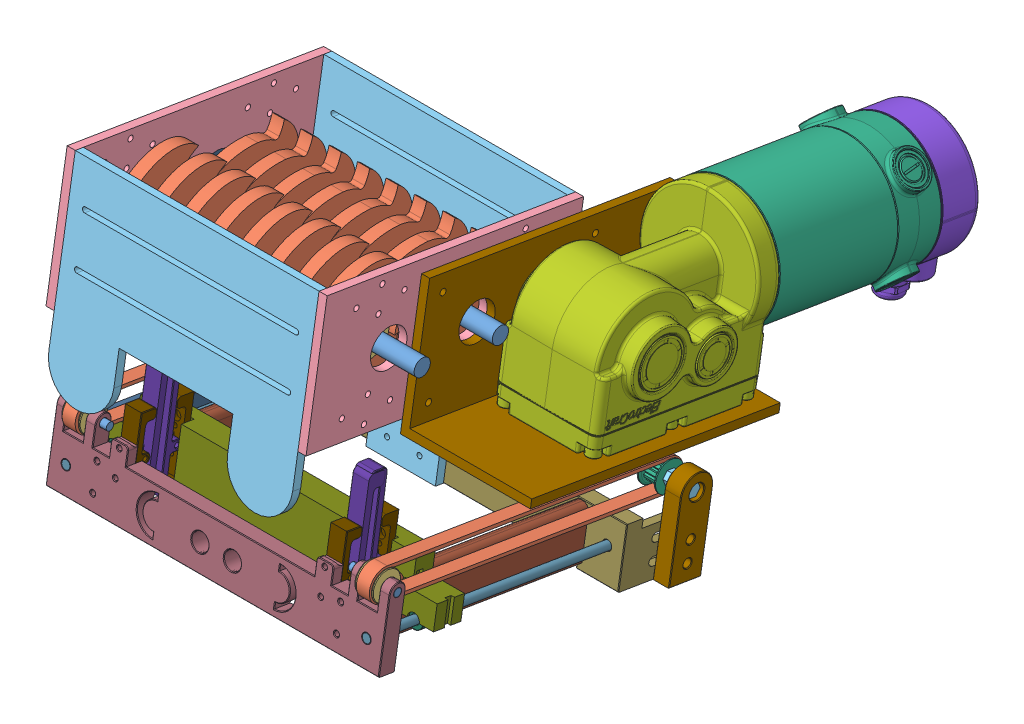
SolidWorks assembly ShredderAssem_fullsize, configuration Default. Lengths in mm.
Overall size (342.26 262.01 457.48).
89 component instances, 30 part files, 28 mates.
Components (placement in the parent):
- shaftassem_fullsize-1: shaftassem_fullsize [Default] at (-192.7659 88.7828 -80.3158) x (1 0 0) z (0 -0.831108 -0.556112) size (254 113.01 112.98)
  - shaft_approx-2: shaft_approx [Default] at (125.6129 231.0581 -203.0005) size (254 12.7 12.7)
  - Blade-9: Blade [Default] at (163.7129 231.0581 -203.0005) x (1 0 0) z (0 0.717916 0.696129) size (9.53 79.05 80.77)
  - grainger-36wy84-1: grainger-36wy84 [Default] at (178.0004 231.0581 -203.0005) x (0 0.857491 -0.514498) z (1 0 0) size (31.74 31.75 9.53)
  - grainger-36wy84-6: grainger-36wy84 [Default] at (200.2254 231.0581 -203.0005) x (0 0.857491 -0.514498) z (1 0 0) size (31.74 31.75 9.53)
  - grainger-36wy84-7: grainger-36wy84 [Default] at (222.4504 231.0581 -203.0005) x (0 0.857491 -0.514498) z (1 0 0) size (31.74 31.75 9.53)
  - grainger-36wy84-8: grainger-36wy84 [Default] at (244.6754 231.0581 -203.0005) x (0 0.857491 -0.514498) z (1 0 0) size (31.74 31.75 9.53)
  - Blade-14: Blade [Default] at (185.9379 231.0581 -203.0005) x (1 0 0) z (0 0.717916 0.696129) size (9.53 79.05 80.77)
  - Blade-15: Blade [Default] at (208.1629 231.0581 -203.0005) x (1 0 0) z (0 0.717916 0.696129) size (9.53 79.05 80.77)
  - Blade-16: Blade [Default] at (230.3879 231.0581 -203.0005) x (1 0 0) z (0 0.717916 0.696129) size (9.53 79.05 80.77)
  - Blade-17: Blade [Default] at (252.6129 231.0581 -203.0005) x (1 0 0) z (0 0.717916 0.696129) size (9.53 79.05 80.77)
  - Blade-18: Blade [Default] at (274.8379 231.0581 -203.0005) x (1 0 0) z (0 0.717916 0.696129) size (9.53 79.05 80.77)
  - Blade-19: Blade [Default] at (297.0629 231.0581 -203.0005) x (1 0 0) z (0 0.717916 0.696129) size (9.53 79.05 80.77)
  - grainger-36wy84-9: grainger-36wy84 [Default] at (266.9004 231.0581 -203.0005) x (0 0.857491 -0.514498) z (1 0 0) size (31.74 31.75 9.53)
  - grainger-36wy84-10: grainger-36wy84 [Default] at (289.1254 231.0581 -203.0005) x (0 0.857491 -0.514498) z (1 0 0) size (31.74 31.75 9.53)
  - grainger-36wy84-11: grainger-36wy84 [Default] at (311.3504 231.0581 -203.0005) x (0 0.857491 -0.514498) z (1 0 0) size (31.74 31.75 9.53)
  - grainger-36wy84-13: grainger-36wy84 [Default] at (333.5754 231.0581 -203.0005) x (0 0.857491 -0.514498) z (1 0 0) size (31.74 31.75 9.53)
  - Blade-21: Blade [Default] at (319.2879 231.0581 -203.0005) x (1 0 0) z (0 0.717916 0.696129) size (9.53 79.05 80.77)
- frontWall(forExcessToothOverlap)-1: frontWall(forExcessToothOverlap) [Default] at (160.6532 55.1224 88.7684) x (0 0.162672 0.98668) z (-1 0 0) size (203.2 221.08 6.35)
- shaftassem_fullsize-2: shaftassem_fullsize [Default] at (310.8723 -109.7477 367.9172) x (-1 0 0) z (0 -0.993255 -0.115948) size (254 113.01 112.98)
  - shaft_approx-2: shaft_approx [Default] at (125.6129 231.0581 -203.0005) size (254 12.7 12.7)
  - Blade-9: Blade [Default] at (163.7129 231.0581 -203.0005) x (1 0 0) z (0 0.717916 0.696129) size (9.53 79.05 80.77)
  - grainger-36wy84-1: grainger-36wy84 [Default] at (178.0004 231.0581 -203.0005) x (0 0.857491 -0.514498) z (1 0 0) size (31.74 31.75 9.53)
  - grainger-36wy84-6: grainger-36wy84 [Default] at (200.2254 231.0581 -203.0005) x (0 0.857491 -0.514498) z (1 0 0) size (31.74 31.75 9.53)
  - grainger-36wy84-7: grainger-36wy84 [Default] at (222.4504 231.0581 -203.0005) x (0 0.857491 -0.514498) z (1 0 0) size (31.74 31.75 9.53)
  - grainger-36wy84-8: grainger-36wy84 [Default] at (244.6754 231.0581 -203.0005) x (0 0.857491 -0.514498) z (1 0 0) size (31.74 31.75 9.53)
  - Blade-14: Blade [Default] at (185.9379 231.0581 -203.0005) x (1 0 0) z (0 0.717916 0.696129) size (9.53 79.05 80.77)
  - Blade-15: Blade [Default] at (208.1629 231.0581 -203.0005) x (1 0 0) z (0 0.717916 0.696129) size (9.53 79.05 80.77)
  - Blade-16: Blade [Default] at (230.3879 231.0581 -203.0005) x (1 0 0) z (0 0.717916 0.696129) size (9.53 79.05 80.77)
  - Blade-17: Blade [Default] at (252.6129 231.0581 -203.0005) x (1 0 0) z (0 0.717916 0.696129) size (9.53 79.05 80.77)
  - Blade-18: Blade [Default] at (274.8379 231.0581 -203.0005) x (1 0 0) z (0 0.717916 0.696129) size (9.53 79.05 80.77)
  - Blade-19: Blade [Default] at (297.0629 231.0581 -203.0005) x (1 0 0) z (0 0.717916 0.696129) size (9.53 79.05 80.77)
  - grainger-36wy84-9: grainger-36wy84 [Default] at (266.9004 231.0581 -203.0005) x (0 0.857491 -0.514498) z (1 0 0) size (31.74 31.75 9.53)
  - grainger-36wy84-10: grainger-36wy84 [Default] at (289.1254 231.0581 -203.0005) x (0 0.857491 -0.514498) z (1 0 0) size (31.74 31.75 9.53)
  - grainger-36wy84-11: grainger-36wy84 [Default] at (311.3504 231.0581 -203.0005) x (0 0.857491 -0.514498) z (1 0 0) size (31.74 31.75 9.53)
  - grainger-36wy84-13: grainger-36wy84 [Default] at (333.5754 231.0581 -203.0005) x (0 0.857491 -0.514498) z (1 0 0) size (31.74 31.75 9.53)
  - Blade-21: Blade [Default] at (319.2879 231.0581 -203.0005) x (1 0 0) z (0 0.717916 0.696129) size (9.53 79.05 80.77)
- frontWall(forExcessToothOverlap)-2: frontWall(forExcessToothOverlap) [Default] at (-42.5468 155.3691 72.2408) x (0 0.162672 0.98668) z (1 0 0) size (203.2 221.08 6.35)
- sideWall_full-1: sideWall_full [Default] at (-36.1968 88.1774 289.2618) x (1 0 0) z (0 0.162672 0.98668) size (190.5 216.5 6.35)
- sideWall_full-2: sideWall_full [Default] at (-36.1968 56.1553 95.0338) x (1 0 0) z (0 0.162672 0.98668) size (190.5 216.5 6.35)
- Motor_Assem-1: Motor_Assem [Default] at (399.8937 297.3505 165.6643) x (0 -0.162672 -0.98668) z (-1 0 0) size (348.06 128.36 160.99)
  - ElectroCraft-MP26-WR-016V24-020-X-1: ElectroCraft-MP26-WR-016V24-020-X [Default] at (174.2174 154.2298 186.8905) size (290.81 122.01 158.49)
    - ElectroCraft-MP26-WR-016V24-020-X_SA_Motor_MPP26-1: ElectroCraft-MP26-WR-016V24-020-X_SA_Motor_MPP26 [Default] at origin size (129.5 93.09 93.09)
    - ElectroCraft-MP26-WR-016V24-020-X_SA_Gearbox_MP_WR_No_Release-1: ElectroCraft-MP26-WR-016V24-020-X_SA_Gearbox_MP_WR_No_Release [Default] at (-88.053 21.463 0) size (133.21 121.76 158.49)
    - ElectroCraft-MP26-WR-016V24-020-X_SA_MTR_Cover_wo_Encoder-Brake-1: ElectroCraft-MP26-WR-016V24-020-X_SA_MTR_Cover_wo_Encoder-Brake [Default] at (129.5 0 0) size (33.63 117.57 92.76)
  - ShredderMotorMount-1: ShredderMotorMount [Default] at (112.1644 229.6928 186.8905) size (196.85 101.6 101.6)
- 5172T16_Metal Gear - 20 Degree Pressure Angle-1: 5172T16_Metal Gear - 20 Degree Pressure Angle [5172T16] at (-55.2468 129.004 224.6092) x (0 0 -1) z (1 0 0) size (53.31 53.31 25.43)
- 5172T16_Metal Gear - 20 Degree Pressure Angle-2: 5172T16_Metal Gear - 20 Degree Pressure Angle [5172T16] at (-55.2468 118.6743 161.9551) x (0 0 -1) z (1 0 0) size (53.31 53.31 25.43)
- Part2^ShredderAssem_fullsize-1: Part2^ShredderAssem_fullsize [Default] at (-42.5468 155.3691 72.2408) x (0 -0.162672 -0.98668) z (-1 0 0) (virtual)
- Full Gantry Assembly COPY-1: Full Gantry Assembly COPY [Default] at (32.3027 -188.1986 -13.0446) x (1 0 0) z (0 0.162672 0.98668) size (316.36 107.99 274.71)
  - Gantry Frame Assembly-1: Gantry Frame Assembly [Default] at (-22.7812 29.2709 55.0882) size (260.35 63.5 254)
    - Frame Side Walls-1: Frame Side Walls [Default] at (-11.2932 98.0952 84.9503) size (12.1 37.5 177.8)
    - Gantry Frame End Piece-1: Gantry Frame End Piece [Default] at (83.9568 98.3952 72.2503) size (260.35 43.18 63.5)
    - Gantry Frame Heating End Piece-1: Gantry Frame Heating End Piece [Default] at (83.9568 98.3952 262.7503) size (260.35 58.42 12.7)
    - Frame Side Walls-2: Frame Side Walls [Default] at (179.2068 98.0952 84.9503) size (12.1 37.5 177.8)
    - 0.25 Diam 9 inch long Linear Rod-1: 0.25 Diam 9 inch long Linear Rod [Default] at (201.4318 98.3952 46.8503) x (0.968537 -0.248869 0) z (0 0 1) size (6.35 6.35 228.6)
    - 0.25 Diam 9 inch long Linear Rod-2: 0.25 Diam 9 inch long Linear Rod [Default] at (-33.5182 98.3952 46.8503) x (0.995745 -0.092157 0) z (0 0 1) size (6.35 6.35 228.6)
  - Gantry Subassembly-1: Gantry Subassembly [Default] at (-16.8456 119.8156 318.0932) size (266.7 99.55 38.74)
    - 60595K11_Fixed Alignment Linear Ball Bearing-1: 60595K11_Fixed Alignment Linear Ball Bearing [60595K11] at (-39.4539 7.8505 -35.6605) size (12.7 12.7 19.05)
    - Gantry Piece-1: Gantry Piece [Default] at (78.0211 25.6305 -35.6605) size (266.7 50.8 22.23)
    - 60595K11_Fixed Alignment Linear Ball Bearing-2: 60595K11_Fixed Alignment Linear Ball Bearing [60595K11] at (195.4961 7.8505 -35.6605) x (0.99266 0.120939 0) z (0 0 1) size (12.7 12.7 19.05)
    - Clip Assembly-1: Clip Assembly [Default] at (45.7541 -13.0009 -33.2659) x (0 0.02134 0.999772) z (-1 0 0) size (28.26 95.92 12.7)
      - Added Clip Piece-1: Added Clip Piece [Default] at (13.6312 56.6752 41.3294) x (0.999405 -0.034486 0) z (0 0 1) size (20.96 95.25 12.7)
      - Attatched Clip Piece-1: Attatched Clip Piece [Default] at (0.3891 41.1725 54.0294) x (-0.999772 0.02134 0) z (0 0 -1) size (12.7 63.5 12.7)
    - Clip Assembly-2: Clip Assembly [Default] at (205.6471 -13.0009 -33.2659) x (0 0.02134 0.999772) z (-1 0 0) size (28.26 95.92 12.7)
      - Added Clip Piece-1: Added Clip Piece [Default] at (13.6312 56.6752 41.3294) x (0.999405 -0.034486 0) z (0 0 1) size (20.96 95.25 12.7)
      - Attatched Clip Piece-1: Attatched Clip Piece [Default] at (0.3891 41.1725 54.0294) x (-0.999772 0.02134 0) z (0 0 -1) size (12.7 63.5 12.7)
  - Clip Assembly-1: Clip Assembly [Default] at (93.7601 105.5448 319.8889) x (0 0.02134 -0.999772) z (1 0 0) size (27.33 95.65 12.7) (flexible)
    - Added Clip Piece-1: Added Clip Piece [Default] at (13.4006 56.7842 41.3294) x (0.999804 -0.019788 0) z (0 0 1) size (20.96 95.25 12.7)
    - Attatched Clip Piece-1: Attatched Clip Piece [Default] at (0.3891 41.1725 54.0294) x (-0.999772 0.02134 0) z (0 0 -1) size (12.7 63.5 12.7)
  - Clip Assembly-2: Clip Assembly [Default] at (-66.7679 105.5448 319.8889) x (0 0.02134 -0.999772) z (1 0 0) size (27.36 95.66 12.7) (flexible)
    - Added Clip Piece-1: Added Clip Piece [Default] at (13.4085 56.7805 41.3294) x (0.999794 -0.020292 0) z (0 0 1) size (20.96 95.25 12.7)
    - Attatched Clip Piece-1: Attatched Clip Piece [Default] at (0.3891 41.1725 54.0294) x (-0.999772 0.02134 0) z (0 0 -1) size (12.7 63.5 12.7)
  - Passive Pulley Axle-1: Passive Pulley Axle [Default] at (-68.9995 160.6862 324.1885) x (0 -0.395908 -0.91829) z (0 -0.91829 0.395908) size (5.85 35.56 5.85)
  - Passive Pulley Axle-2: Passive Pulley Axle [Default] at (191.3505 160.6862 324.1885) x (0 -0.802318 -0.596897) z (0 0.596897 -0.802318) size (5.85 35.56 5.85)
  - Pulley and Belt Assembly-1: Pulley and Belt Assembly [Default] at (-262.393 22.4987 259.1542) x (0 0 -1) z (1 0 0) size (254.91 31.32 266.45) (flexible)
    - 20 Inch Belt-1: 20 Inch Belt [Default] at (47.0039 138.1875 203.6424) size (248.21 24.13 10.16)
    - Belt Idler Pulley-1: Belt Idler Pulley [6495K744] at (-65.0343 138.1875 212.2657) x (0.999956 -0.009357 0) z (0 0 1) size (22.23 22.23 14.3)
    - Belt Idler Pulley Coupler-1: Belt Idler Pulley Coupler [6495K744] at (159.0421 138.1875 205.9411) x (0.5 0.866025 0) z (0 0 -1) size (22.23 22.23 19.13)
    - Hexshaft Motor Drive Axle-1: Hexshaft Motor Drive Axle [Default] at (159.2153 138.1875 463.5733) x (0.5 -0.866025 0) z (0.866025 0.5 0) size (11 254 9.53)
    - Belt Idler Pulley Hex Hole-1: Belt Idler Pulley Hex Hole [6495K744] at (159.2153 138.1875 441.1959) x (-0.5 -0.866025 0) z (0 0 1) size (22.23 22.23 14.3)
    - Belt Idler Pulley-2: Belt Idler Pulley [6495K744] at (-64.8611 138.1875 441.1959) x (0.643871 0.765134 0) z (0 0 1) size (22.23 22.23 14.3)
    - 20 Inch Belt-2: 20 Inch Belt [Default] at (47.1771 138.1875 443.4946) x (1 0 0) z (0 0 -1) size (248.21 24.13 10.16)
  - Stepper Mount and Tensioner-1: Stepper Mount and Tensioner [Default] at (-96.2784 207.8478 159.2914) x (1 0 0) z (0 -0.924225 0.381849) size (61.75 74.03 91.46)
    - Stepper Motor-1: Stepper Motor [Default] at (4.7189 -72.7035 20.9904) x (0 -0.924225 -0.381849) z (1 0 0) size (42.5 46.5 61.75)
    - Stepper Motor Mount-2: Stepper Motor Mount [Default] at (27.2789 -72.7035 20.9904) x (-1 0 0) z (0 -0.924225 -0.381849) size (29.21 76.08 48.66)
  - Opposite tensioner-1: Opposite tensioner [Default] at (191.3505 103.5362 112.6389) x (0 0 -1) z (1 0 0) size (25.4 69.85 12.7)
  - Spring Board-2: Spring Board [Default] at (-11.2145 108.6162 299.6968) x (1 0 0) z (0 -1 0) size (144.78 50.8 38.1) (hidden)
  - Part4^Full Gantry Assembly COPY-1: Part4^Full Gantry Assembly COPY [Default] at (61.1755 127.6662 140.0385) size (5.08 42.18 177.8) (virtual)
Mates (geometry in assembly coordinates):
- Concentric1: concentric anti-aligned: circle of shaftassem_fullsize-1/shaft_approx-2; circle of frontWall(forExcessToothOverlap)-1
- Concentric2: concentric aligned: cylinder of frontWall(forExcessToothOverlap)-1 through (201.0643 118.6743 161.9551) axis (-1 0 0) radius 14.2875; circle of shaftassem_fullsize-2/shaft_approx-2
- Distance6: distance = 1.5875 mm anti-aligned: plane of shaftassem_fullsize-1/Blade-21 through (126.5219 129.004 224.6092) normal (-1 0 0); plane of shaftassem_fullsize-2/Blade-14 through (124.9344 118.6743 161.9551) normal (1 0 0)
- Distance8: distance = 7.1437 mm anti-aligned: plane of shaftassem_fullsize-2/Blade-9 through (147.1594 118.6743 161.9551) normal (1 0 0); plane of frontWall(forExcessToothOverlap)-1 through (154.3032 55.1224 88.7684) normal (-1 0 0)
- Distance9: distance = 8.7312 mm anti-aligned: plane of shaftassem_fullsize-2/grainger-36wy84-13 through (-27.4656 118.6743 161.9551) normal (-1 0 0); plane of frontWall(forExcessToothOverlap)-2 through (-36.1968 155.3691 72.2408) normal (1 0 0)
- Concentric3: concentric anti-aligned: cylinder of shaftassem_fullsize-1/shaft_approx-2 through (186.8469 129.004 224.6092) axis (-1 0 0) radius 6.35; cylinder of frontWall(forExcessToothOverlap)-2 through (-82.958 129.004 224.6092) axis (1 0 0) radius 14.2875
- Concentric4: concentric aligned: cylinder of shaftassem_fullsize-2/shaft_approx-2 through (-68.7406 118.6743 161.9551) axis (1 0 0) radius 6.35; cylinder of frontWall(forExcessToothOverlap)-2 through (-82.958 118.6743 161.9551) axis (1 0 0) radius 14.2875
- Coincident1: coincident anti-aligned: plane of frontWall(forExcessToothOverlap)-2 through (-36.1968 155.3691 72.2408) normal (1 0 0); plane of sideWall_full-2 through (-36.1968 156.402 78.5063) normal (-1 0 0)
- Coincident2: coincident aligned: plane of frontWall(forExcessToothOverlap)-2 through (-36.1968 155.3691 72.2408) normal (0 0.98668 -0.162672); plane of sideWall_full-2 through (-36.1968 156.402 78.5063) normal (0 0.98668 -0.162672)
- Coincident3: coincident aligned: plane of frontWall(forExcessToothOverlap)-2 through (-36.1968 155.3691 72.2408) normal (0 -0.162672 -0.98668); plane of sideWall_full-2 through (-36.1968 155.3691 72.2408) normal (0 -0.162672 -0.98668)
- Coincident4: coincident aligned: plane of frontWall(forExcessToothOverlap)-2 through (-36.1968 188.4241 272.7343) normal (0 0.162672 0.98668); plane of sideWall_full-1 through (-36.1968 188.4241 272.7343) normal (0 0.162672 0.98668)
- Coincident5: coincident anti-aligned: plane of frontWall(forExcessToothOverlap)-2 through (-36.1968 155.3691 72.2408) normal (1 0 0); plane of sideWall_full-1 through (-36.1968 188.4241 272.7343) normal (-1 0 0)
- Coincident7: coincident anti-aligned: plane of frontWall(forExcessToothOverlap)-1 through (160.6532 55.1224 88.7684) normal (1 0 0); plane of Motor_Assem-1/ShredderMotorMount-1 through (160.6532 34.3141 21.2641) normal (-1 0 0)
- Concentric5: concentric anti-aligned: circle of frontWall(forExcessToothOverlap)-1; circle of Motor_Assem-1/ShredderMotorMount-1
- Concentric6: concentric anti-aligned: circle of frontWall(forExcessToothOverlap)-1; circle of Motor_Assem-1/ShredderMotorMount-1
- Coincident19: coincident anti-aligned: plane of frontWall(forExcessToothOverlap)-2 through (-42.5468 155.3691 72.2408) normal (-1 0 0); plane of 5172T16_Metal Gear - 20 Degree Pressure Angle-1 through (-42.5468 129.004 224.6092) normal (1 0 0)
- Concentric7: concentric anti-aligned: cylinder of shaftassem_fullsize-1/shaft_approx-2 through (186.8469 129.004 224.6092) axis (-1 0 0) radius 6.35; cylinder of 5172T16_Metal Gear - 20 Degree Pressure Angle-1 through (-42.5468 129.004 224.6092) axis (1 0 0) radius 6.35
- Coincident20: coincident anti-aligned: plane of frontWall(forExcessToothOverlap)-2 through (-42.5468 155.3691 72.2408) normal (-1 0 0); plane of 5172T16_Metal Gear - 20 Degree Pressure Angle-2 through (-42.5468 118.6743 161.9551) normal (1 0 0)
- Concentric8: concentric aligned: cylinder of shaftassem_fullsize-2/shaft_approx-2 through (-68.7406 118.6743 161.9551) axis (1 0 0) radius 6.35; cylinder of 5172T16_Metal Gear - 20 Degree Pressure Angle-2 through (-42.5468 118.6743 161.9551) axis (1 0 0) radius 6.35
- InPlace1: in place: plane of frontWall(forExcessToothOverlap)-2 through (-42.5468 155.3691 72.2408) normal (-1 0 0); plane of ? through (-42.5468 0 0) normal (-1 0 0); moOrthogonalPlaneRef_w of frontWall(forExcessToothOverlap)-2 through (-42.5468 155.3691 72.2408) normal (-1 0 0); plane of ? through (-42.5468 0 0) normal (0 1 0); plane of frontWall(forExcessToothOverlap)-2 through (-42.5468 155.3691 72.2408) normal (-1 0 0); plane of ? through (-42.5468 0 0) normal (0 0 1); plane of frontWall(forExcessToothOverlap)-2 through (-42.5468 155.3691 72.2408) normal (-1 0 0); unknown of Part2^ShredderAssem_fullsize-1
- Coincident21: coincident aligned: plane of frontWall(forExcessToothOverlap)-2; plane of Part2^ShredderAssem_fullsize-1
- Coincident22: coincident aligned: moOrthogonalPlaneRef_w of frontWall(forExcessToothOverlap)-2 through (-42.5468 155.3691 72.2408) normal (0 -0.98668 0.162672); plane of Part2^ShredderAssem_fullsize-1 through (-42.5468 155.3691 72.2408) normal (0 -0.98668 0.162672)
- Coincident23: coincident anti-aligned: moOrthogonalPlaneRef_w of frontWall(forExcessToothOverlap)-2 through (-42.5468 155.3691 72.2408) normal (0 0.162672 0.98668); plane of Part2^ShredderAssem_fullsize-1 through (-42.5468 155.3691 72.2408) normal (0 -0.162672 -0.98668)
- Parallel6: parallel aligned: plane of sideWall_full-1 through (-36.1968 188.4241 272.7343) normal (0 0.162672 0.98668); plane of Full Gantry Assembly COPY-1/Gantry Frame Assembly-1/Gantry Frame Heating End Piece-1 through (9.1502 20.3575 287.5717) normal (0 0.162672 0.98668)
- Parallel7: parallel aligned: plane of frontWall(forExcessToothOverlap)-2 through (-42.5468 155.3691 72.2408) normal (-1 0 0); plane of Full Gantry Assembly COPY-1/Part4^Full Gantry Assembly COPY-1 through (-36.1968 14.6847 318.6938) normal (-1 0 0)
- Coincident26: coincident anti-aligned: plane of frontWall(forExcessToothOverlap)-2 through (-36.1968 155.3691 72.2408) normal (1 0 0); plane of Full Gantry Assembly COPY-1/Part4^Full Gantry Assembly COPY-1 through (-36.1968 14.6847 318.6938) normal (-1 0 0)
- Distance11: distance = 12.7 mm aligned: plane of Full Gantry Assembly COPY-1/Gantry Frame Assembly-1/Gantry Frame Heating End Piece-1 through (9.1502 20.3575 287.5717) normal (0 0.162672 0.98668); plane of sideWall_full-1 through (-36.1968 188.4241 272.7343) normal (0 0.162672 0.98668)
- Coincident29: coincident aligned: plane of frontWall(forExcessToothOverlap)-2 through (-42.5468 -62.7678 108.2047) normal (0 -0.98668 0.162672); plane of Full Gantry Assembly COPY-1/Part4^Full Gantry Assembly COPY-1 through (-36.1968 -26.9335 325.5554) normal (0 -0.98668 0.162672)
